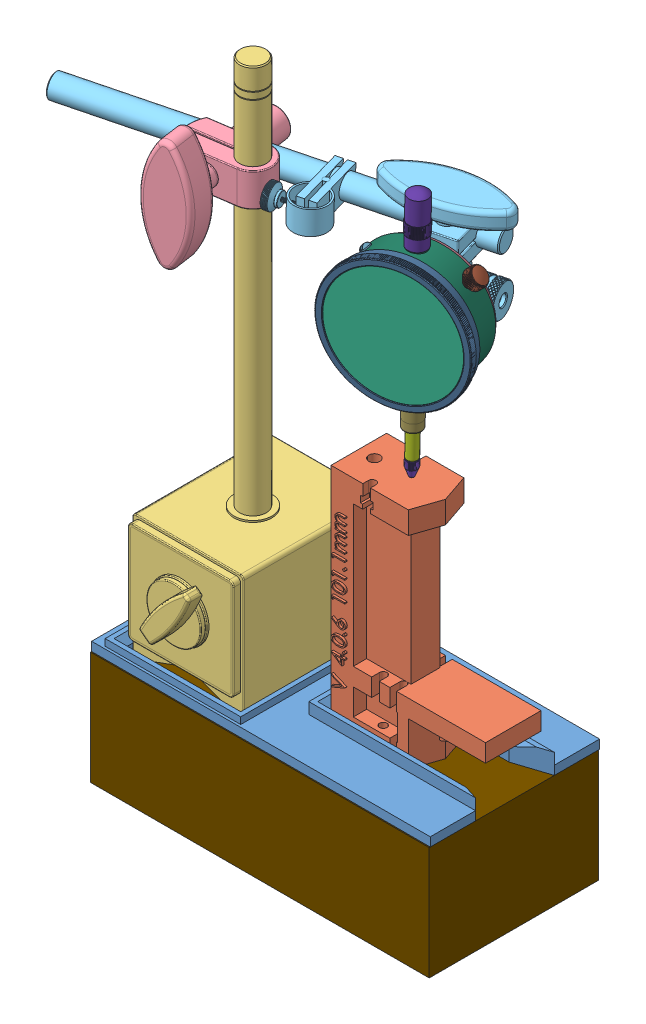
SolidWorks assembly pillar qc v2, configuration Default. Lengths in mm.
Overall size (198.03 281.55 84.37).
23 component instances, 18 part files, 9 mates.
Components (placement in the parent):
- base and pillar jig-1: base and pillar jig [Default] at origin size (152.4 9 76.2)
- shorter pillar 4.0.6 101.1mm-1: shorter pillar 4.0.6 101.1mm [Default] at (31.2 50.55 0.25) size (69.51 101.1 26)
- dial on clamp-2: dial on clamp [Default] at (-41.1937 27.4955 0.4993) size (184.57 230.75 84.37)
  - base-1: base [2310A15] at origin size (50.01 230.75 74.55)
  - nob-1: nob [2310A15] at (0 99.6315 0) x (0.989595 0 -0.143884) z (0.143884 0 0.989595) size (35.61 50.2 58.28)
  - arm-1: arm [2310A15] at (-110.3908 171.5709 0.6957) x (0.022424 0.999742 -0.003719) z (-0.273737 0.002562 -0.961801) size (45.9 172.8 31.52)
  - Dial indicator - Mitutoyo NO.2046.step-1: Dial indicator - Mitutoyo NO.2046.step [Default] at (69.5876 137.9526 -7.5391) x (0.961543 -0.022586 -0.273724) z (0.022152 0.999744 -0.004678) size (57.45 42.2 113.3)
    - Glass.step-1: Glass.step [Default] at (0 -18.65 0) x (0 0 1) z (-1 0 0) size (51.5 1.75 51.5)
    - Shaft.step-1: Shaft.step [Default] at (0 -5.75 29) size (6 6 90.9)
    - Tip.step-1: Tip.step [Default] at (0 -5.75 -52.3) size (5 5 12.5)
    - Back screw.step-1: Back screw.step [Default] at (16.2988 -3.2 -16.2988) x (0.707107 0 0.707107) z (0 1 0) size (3 3 5)
    - Dial.step-1: Dial.step [Default] at (0 -15.1 0) size (57.45 8.05 57.45)
    - Back screw.step-2: Back screw.step [Default] at (-16.2988 -3.2 -16.2988) x (0.707107 0 -0.707107) z (0 1 0) size (3 3 5)
    - Back screw.step-3: Back screw.step [Default] at (-16.2988 -3.2 16.2988) x (0.707107 0 0.707107) z (0 1 0) size (3 3 5)
    - Knurled screw.step-1: Knurled screw.step [Default] at (15.9356 -5.75 15.9356) x (0.707107 0 -0.707107) z (0.707107 0 0.707107) size (8.17 8.17 10.7)
    - Stem.step-1: Stem.step [Default] at (0 -5.85 -45.0423) size (7.9 7.9 24)
    - Back screw.step-4: Back screw.step [Default] at (16.2988 -3.2 16.2988) x (-0.707107 0 0.707107) z (0 1 0) size (3 3 5)
    - Back cover and lug.step-1: Back cover and lug.step [Default] x (1 0 0) z (0 0 -1) size (50.2 21.55 50.2)
    - M2.5x3.7.step-1: M2.5x3.7.step [Default] at (-19.6479 -5.75 19.6479) x (-0.707107 0 -0.707107) z (-0.707107 0 0.707107) size (4.4 4.4 5.4)
    - Case.step-1: Case.step [Default] at origin size (52 15.1 55.04)
    - Long pointer.step-1: Long pointer.step [Default] at (0 -18.6 0) x (0.431825 0 0.901957) z (-0.901957 0 0.431825) size (3.8 6.56 25.9)
    - Cover knob.step-1: Cover knob.step [Default] at (0 -5.75 26.5) size (8.99 8.99 22)
- 1388K806_Ground Low-Carbon Steel Sheet-1: 1388K806_Ground Low-Carbon Steel Sheet [1388K806] at (0 -25.4 0.4662) x (0 0 -1) z (1 0 0) size (76.2 50.8 152.4)
Mates (geometry in assembly coordinates):
- Coincident4: coincident aligned: plane of base and pillar jig-1 through (0 0 0) normal (0 -1 0); plane of shorter pillar 4.0.6 101.1mm-1 through (56.2 0 12.75) normal (0 -1 0)
- Coincident5: coincident anti-aligned: plane of base and pillar jig-1 through (76.2 0 12.75) normal (0 0 -1); plane of shorter pillar 4.0.6 101.1mm-1 through (31.2 50.55 12.75) normal (0 0 1)
- Parallel1: parallel anti-aligned: plane of base and pillar jig-1 through (76.2 0 -12.75) normal (0 0 1); plane of shorter pillar 4.0.6 101.1mm-1 through (31.2 50.55 -12.25) normal (0 0 -1)
- Coincident8: coincident aligned: plane of base and pillar jig-1 through (0 0 0) normal (0 -1 0); plane of dial on clamp-2/base-1 through (-66.2 0 29.7487) normal (0 -1 0)
- Coincident9: coincident anti-aligned: plane of base and pillar jig-1 through (-66.2 0 -32) normal (0 0 1); plane of dial on clamp-2/base-1 through (-41.1937 27.4955 -32) normal (0 0 -1)
- Coincident10: coincident anti-aligned: plane of base and pillar jig-1 through (-66.2 0 -32) normal (1 0 0); plane of dial on clamp-2/base-1 through (-66.2 54.991 29.7487) normal (-1 0 0)
- Coincident11: coincident anti-aligned: plane of base and pillar jig-1 through (6.2 0 -12.75) normal (1 0 0); plane of shorter pillar 4.0.6 101.1mm-1 through (6.2 0 12.75) normal (-1 0 0)
- Coincident12: coincident aligned: plane of base and pillar jig-1 through (-76.2 4 -38.1) normal (-1 0 0); plane of 1388K806_Ground Low-Carbon Steel Sheet-1 through (-76.2 -25.4 0.4662) normal (-1 0 0)
- Coincident13: coincident anti-aligned: plane of base and pillar jig-1 through (0 0 0) normal (0 -1 0); plane of 1388K806_Ground Low-Carbon Steel Sheet-1 through (76.2 0 -37.6338) normal (0 1 0)
